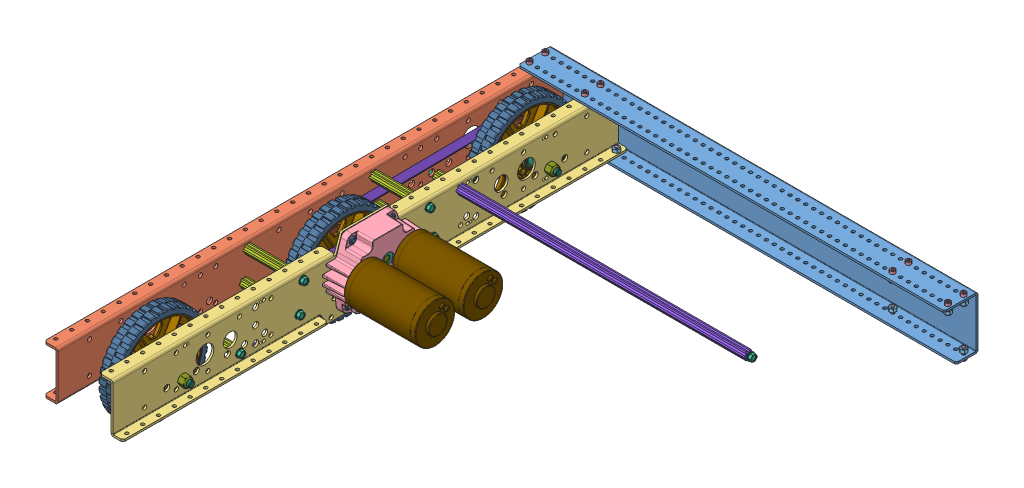
SolidWorks assembly AM14U4 Long Half, configuration Default. Lengths in mm.
Overall size (686.9 159.29 816.74).
156 component instances, 36 part files, 34 mates.
Components (placement in the parent):
- AM14U4 Long Frame Half-1: AM14U4 Long Frame Half [Default] at (226.8656 49.3843 -371.735) size (686.9 116.33 816.74)
  - am-3920 AM14U4 End Plate Long-1: am-3920 AM14U4 End Plate Long [Default] at (-787.4 -81.407 -3.175) x (1 0 0) z (0 -1 0) size (685.8 53.98 84.58)
  - am-3921 AM14U4 Outside Plate-2: am-3921 AM14U4 Outside Plate [Default] at (-666.75 -77.216 813.562) x (0 0 -1) z (0 -1 0) size (812.8 22.23 77.72)
  - am-3922 AM14U4 Inside Plate-1: am-3922 AM14U4 Inside Plate [Default] at (-577.85 -77.216 813.562) x (0 0 -1) z (0 -1 0) size (812.8 38.1 116.33)
  - am-1002 and am-1042 10-32 x 0500 and Nylock Nut Assembly-7: am-1002 and am-1042 10-32 x 0500 and Nylock Nut Assembly [Default] at (-9.8821 -6.6363 9.8132) x (0 -1 0) z (0 0 1) size (17.53 13.8 13)
    - 10-32x0500_shcs-1: 10-32x0500_shcs [HX-SHCS 0.19-32x1.375x1-C] at (-11.4623 3.5321 3.6488) size (17.53 7.94 7.94)
    - 10-32 Nylock Nut 1-1: 10-32 Nylock Nut 1 [90631A411] at (-0.0323 3.5321 3.6488) x (0 0.381849 -0.924225) z (0 -0.924225 -0.381849) size (9.53 6.11 11)
  - am-1002 and am-1042 10-32 x 0500 and Nylock Nut Assembly-8: am-1002 and am-1042 10-32 x 0500 and Nylock Nut Assembly [Default] at (-9.8821 -6.6363 35.2132) x (0 -1 0) z (0 0 1) size (17.53 13.8 13)
    - 10-32x0500_shcs-1: 10-32x0500_shcs [HX-SHCS 0.19-32x1.375x1-C] at (-11.4623 3.5321 3.6488) size (17.53 7.94 7.94)
    - 10-32 Nylock Nut 1-1: 10-32 Nylock Nut 1 [90631A411] at (-0.0323 3.5321 3.6488) x (0 0.381849 -0.924225) z (0 -0.924225 -0.381849) size (9.53 6.11 11)
  - am-1002 and am-1042 10-32 x 0500 and Nylock Nut Assembly-9: am-1002 and am-1042 10-32 x 0500 and Nylock Nut Assembly [Default] at (-2.8179 -77.9457 9.8132) x (0 1 0) z (0 0 1) size (17.53 13.8 13)
    - 10-32x0500_shcs-1: 10-32x0500_shcs [HX-SHCS 0.19-32x1.375x1-C] at (-11.4623 3.5321 3.6488) size (17.53 7.94 7.94)
    - 10-32 Nylock Nut 1-1: 10-32 Nylock Nut 1 [90631A411] at (-0.0323 3.5321 3.6488) x (0 0.381849 -0.924225) z (0 -0.924225 -0.381849) size (9.53 6.11 11)
  - am-1002 and am-1042 10-32 x 0500 and Nylock Nut Assembly-10: am-1002 and am-1042 10-32 x 0500 and Nylock Nut Assembly [Default] at (-98.7821 -6.6363 9.8132) x (0 -1 0) z (0 0 1) size (17.53 13.8 13)
    - 10-32x0500_shcs-1: 10-32x0500_shcs [HX-SHCS 0.19-32x1.375x1-C] at (-11.4623 3.5321 3.6488) size (17.53 7.94 7.94)
    - 10-32 Nylock Nut 1-1: 10-32 Nylock Nut 1 [90631A411] at (-0.0323 3.5321 3.6488) x (0 0.381849 -0.924225) z (0 -0.924225 -0.381849) size (9.53 6.11 11)
  - am-1002 and am-1042 10-32 x 0500 and Nylock Nut Assembly-11: am-1002 and am-1042 10-32 x 0500 and Nylock Nut Assembly [Default] at (-98.7821 -6.6363 35.2132) x (0 -1 0) z (0 0 1) size (17.53 13.8 13)
    - 10-32x0500_shcs-1: 10-32x0500_shcs [HX-SHCS 0.19-32x1.375x1-C] at (-11.4623 3.5321 3.6488) size (17.53 7.94 7.94)
    - 10-32 Nylock Nut 1-1: 10-32 Nylock Nut 1 [90631A411] at (-0.0323 3.5321 3.6488) x (0 0.381849 -0.924225) z (0 -0.924225 -0.381849) size (9.53 6.11 11)
  - am-1002 and am-1042 10-32 x 0500 and Nylock Nut Assembly-12: am-1002 and am-1042 10-32 x 0500 and Nylock Nut Assembly [Default] at (-117.1179 -77.9457 9.8132) x (0 1 0) z (0 0 1) size (17.53 13.8 13)
    - 10-32x0500_shcs-1: 10-32x0500_shcs [HX-SHCS 0.19-32x1.375x1-C] at (-11.4623 3.5321 3.6488) size (17.53 7.94 7.94)
    - 10-32 Nylock Nut 1-1: 10-32 Nylock Nut 1 [90631A411] at (-0.0323 3.5321 3.6488) x (0 0.381849 -0.924225) z (0 -0.924225 -0.381849) size (9.53 6.11 11)
  - FHTS 0.25-20-0.75-1: FHTS 0.25-20-0.75 [FHTS 0.25-20-G-0.75-C] at (-574.675 -59.6687 514.6875) x (-1 0 0) z (0 0.924225 0.381849) size (24.64 12.19 12.19)
  - FHTS 0.25-20-0.75-2: FHTS 0.25-20-0.75 [FHTS 0.25-20-G-0.75-C] at (-574.675 -59.6687 299.6365) x (-1 0 0) z (0 0.924225 0.381849) size (24.64 12.19 12.19)
  - FHTS 0.25-20-0.75-3: FHTS 0.25-20-0.75 [FHTS 0.25-20-G-0.75-C] at (-666.75 -59.6687 299.6365) x (1 0 0) z (0 -0.98696 0.160968) size (24.64 12.19 12.19)
  - FHTS 0.25-20-0.75-4: FHTS 0.25-20-0.75 [FHTS 0.25-20-G-0.75-C] at (-666.75 -59.6687 514.6875) size (24.64 12.19 12.19)
  - FHTS 0.25-20-0.75-5: FHTS 0.25-20-0.75 [FHTS 0.25-20-G-0.75-C] at (-666.75 -65.786 610.362) size (24.64 12.19 12.19)
  - FHTS 0.25-20-0.75-6: FHTS 0.25-20-0.75 [FHTS 0.25-20-G-0.75-C] at (-666.75 -65.786 203.962) size (24.64 12.19 12.19)
  - FHTS 0.25-20-0.75-7: FHTS 0.25-20-0.75 [FHTS 0.25-20-G-0.75-C] at (-574.675 -65.786 203.962) x (-1 0 0) z (0 0.924225 0.381849) size (24.64 12.19 12.19)
  - FHTS 0.25-20-0.75-8: FHTS 0.25-20-0.75 [FHTS 0.25-20-G-0.75-C] at (-574.675 -65.786 610.362) x (-1 0 0) z (0 0.924225 0.381849) size (24.64 12.19 12.19)
  - 3.375in Churro-1: 3.375in Churro [Default] at (-577.85 -65.786 610.362) x (0 0 1) z (-1 0 0) size (14.66 12.7 85.72)
  - 3.375in Churro-2: 3.375in Churro [Default] at (-577.85 -59.6687 514.6875) x (0 0 1) z (-1 0 0) size (14.66 12.7 85.72)
  - 3.375in Churro-3: 3.375in Churro [Default] at (-577.85 -59.6687 299.6365) x (0 0 1) z (-1 0 0) size (14.66 12.7 85.72)
  - 3.375in Churro-4: 3.375in Churro [Default] at (-577.85 -65.786 203.962) x (0 0 1) z (-1 0 0) size (14.66 12.7 85.72)
  - FHTS 0.25-20-0.75-10: FHTS 0.25-20-0.75 [FHTS 0.25-20-G-0.75-C] at (-107.95 -14.986 254.762) x (-1 0 0) z (0 0.924225 0.381849) size (24.64 12.19 12.19)
  - am-1002 and am-1042 10-32 x 0500 and Nylock Nut Assembly-13: am-1002 and am-1042 10-32 x 0500 and Nylock Nut Assembly [Default] at (-682.9821 -6.6363 35.2132) x (0 -1 0) z (0 0 1) size (17.53 13.8 13)
    - 10-32x0500_shcs-1: 10-32x0500_shcs [HX-SHCS 0.19-32x1.375x1-C] at (-11.4623 3.5321 3.6488) size (17.53 7.94 7.94)
    - 10-32 Nylock Nut 1-1: 10-32 Nylock Nut 1 [90631A411] at (-0.0323 3.5321 3.6488) x (0 0.381849 -0.924225) z (0 -0.924225 -0.381849) size (9.53 6.11 11)
  - am-1002 and am-1042 10-32 x 0500 and Nylock Nut Assembly-14: am-1002 and am-1042 10-32 x 0500 and Nylock Nut Assembly [Default] at (-682.9821 -6.6363 9.8132) x (0 -1 0) z (0 0 1) size (17.53 13.8 13)
    - 10-32x0500_shcs-1: 10-32x0500_shcs [HX-SHCS 0.19-32x1.375x1-C] at (-11.4623 3.5321 3.6488) size (17.53 7.94 7.94)
    - 10-32 Nylock Nut 1-1: 10-32 Nylock Nut 1 [90631A411] at (-0.0323 3.5321 3.6488) x (0 0.381849 -0.924225) z (0 -0.924225 -0.381849) size (9.53 6.11 11)
  - am-1002 and am-1042 10-32 x 0500 and Nylock Nut Assembly-15: am-1002 and am-1042 10-32 x 0500 and Nylock Nut Assembly [Default] at (-594.0821 -6.6363 35.2132) x (0 -1 0) z (0 0 1) size (17.53 13.8 13)
    - 10-32x0500_shcs-1: 10-32x0500_shcs [HX-SHCS 0.19-32x1.375x1-C] at (-11.4623 3.5321 3.6488) size (17.53 7.94 7.94)
    - 10-32 Nylock Nut 1-1: 10-32 Nylock Nut 1 [90631A411] at (-0.0323 3.5321 3.6488) x (0 0.381849 -0.924225) z (0 -0.924225 -0.381849) size (9.53 6.11 11)
  - am-1002 and am-1042 10-32 x 0500 and Nylock Nut Assembly-16: am-1002 and am-1042 10-32 x 0500 and Nylock Nut Assembly [Default] at (-594.0821 -6.6363 9.8132) x (0 -1 0) z (0 0 1) size (17.53 13.8 13)
    - 10-32x0500_shcs-1: 10-32x0500_shcs [HX-SHCS 0.19-32x1.375x1-C] at (-11.4623 3.5321 3.6488) size (17.53 7.94 7.94)
    - 10-32 Nylock Nut 1-1: 10-32 Nylock Nut 1 [90631A411] at (-0.0323 3.5321 3.6488) x (0 0.381849 -0.924225) z (0 -0.924225 -0.381849) size (9.53 6.11 11)
  - am-1002 and am-1042 10-32 x 0500 and Nylock Nut Assembly-17: am-1002 and am-1042 10-32 x 0500 and Nylock Nut Assembly [Default] at (-561.6179 -77.9457 9.8132) x (0 1 0) z (0 0 1) size (17.53 13.8 13)
    - 10-32x0500_shcs-1: 10-32x0500_shcs [HX-SHCS 0.19-32x1.375x1-C] at (-11.4623 3.5321 3.6488) size (17.53 7.94 7.94)
    - 10-32 Nylock Nut 1-1: 10-32 Nylock Nut 1 [90631A411] at (-0.0323 3.5321 3.6488) x (0 0.381849 -0.924225) z (0 -0.924225 -0.381849) size (9.53 6.11 11)
  - am-1002 and am-1042 10-32 x 0500 and Nylock Nut Assembly-18: am-1002 and am-1042 10-32 x 0500 and Nylock Nut Assembly [Default] at (-675.9179 -77.9457 9.8132) x (0 1 0) z (0 0 1) size (17.53 13.8 13)
    - 10-32x0500_shcs-1: 10-32x0500_shcs [HX-SHCS 0.19-32x1.375x1-C] at (-11.4623 3.5321 3.6488) size (17.53 7.94 7.94)
    - 10-32 Nylock Nut 1-1: 10-32 Nylock Nut 1 [90631A411] at (-0.0323 3.5321 3.6488) x (0 0.381849 -0.924225) z (0 -0.924225 -0.381849) size (9.53 6.11 11)
  - 18.250in Churro-1: 18.250in Churro [Default] at (-342.9 -14.986 254.762) x (0 0 1) z (-1 0 0) size (14.66 12.7 463.55)
  - FHTS 0.25-20-0.75-11: FHTS 0.25-20-0.75 [FHTS 0.25-20-G-0.75-C] at (-577.85 -14.986 254.762) size (24.64 12.19 12.19)
  - 3.375in Churro-5: 3.375in Churro [Default] at (-663.575 -14.986 305.562) x (0 0.866025 0.5) z (1 0 0) size (14.66 12.7 85.72)
  - FHTS 0.25-20-0.75-12: FHTS 0.25-20-0.75 [FHTS 0.25-20-G-0.75-C] at (-666.75 -14.986 305.562) x (1 0 0) z (0 -0.98696 0.160968) size (24.64 12.19 12.19)
  - FHTS 0.25-20-0.75-14: FHTS 0.25-20-0.75 [FHTS 0.25-20-G-0.75-C] at (-574.675 -14.986 305.562) x (-1 0 0) z (0 0.924225 0.381849) size (24.64 12.19 12.19)
  - FHTS 0.25-20-0.75-15: FHTS 0.25-20-0.75 [FHTS 0.25-20-G-0.75-C] at (-574.675 -14.986 508.762) x (-1 0 0) z (0 0.924225 0.381849) size (24.64 12.19 12.19)
  - 3.375in Churro-6: 3.375in Churro [Default] at (-663.575 -14.986 508.762) x (0 0.866025 0.5) z (1 0 0) size (14.66 12.7 85.72)
  - FHTS 0.25-20-0.75-16: FHTS 0.25-20-0.75 [FHTS 0.25-20-G-0.75-C] at (-666.75 -14.986 508.762) size (24.64 12.19 12.19)
- 6 HiGrip with bearings, pulleys and spacers-1: 6 HiGrip with bearings, pulleys and spacers [Default] at (-425.4709 -83.8657 198.1055) size (85.56 152.4 152.4)
  - 6 HiGrip Asm Rev II-1: 6 HiGrip Asm Rev II [Default] at (83.7987 67.439 110.9939) size (35.05 152.4 152.4)
    - 6 wheel Rev 4-1: 6 wheel Rev 4 [Default] at (-52.6446 9.4231 21.378) size (35.05 132.08 132.08)
    - 6 wheel tread II-1: 6 wheel tread II [Default] at (-65.3446 9.4231 21.378) x (0 0 -1) z (1 0 0) size (152.4 152.4 25.58)
  - 42 tooth HTD Pulley half 2014-1: 42 tooth HTD Pulley half 2014 [Default] at (47.6006 76.862 132.3719) x (1 0 0) z (0 -0.5 0.866025) size (13 74.23 74.23)
  - 42 tooth HTD Pulley half 2014-2: 42 tooth HTD Pulley half 2014 [Default] at (64.263 76.862 132.3719) x (-1 0 0) z (0 -0.499927 0.866067) size (13 74.23 74.23)
  - 1614Z Bearing-1: 1614Z Bearing [Default] at (62.612 76.862 132.3719) x (0 -0.157148 -0.987575) z (-1 0 0) size (28.57 28.57 9.53)
  - 10-24 Hex Washer Rolling x 1.25-1: 10-24 Hex Washer Rolling x 1.25 [93882A213] at (63.247 76.8605 108.5602) x (0 0 -1) z (1 0 0) size (10.52 10.52 35.59)
  - 10-24 Hex Washer Rolling x 1.25-2: 10-24 Hex Washer Rolling x 1.25 [93882A213] at (63.247 97.4833 120.4656) x (0 0 -1) z (1 0 0) size (10.52 10.52 35.59)
  - 10-24 Hex Washer Rolling x 1.25-3: 10-24 Hex Washer Rolling x 1.25 [93882A213] at (63.247 56.2398 144.2799) x (0 0 -1) z (1 0 0) size (10.52 10.52 35.59)
  - 10-24 Hex Washer Rolling x 1.25-4: 10-24 Hex Washer Rolling x 1.25 [93882A213] at (63.247 76.8625 156.1852) x (0 -0.95788 -0.287168) z (1 0 0) size (10.52 10.52 35.59)
  - 10-24 Hex Washer Rolling x 1.25-5: 10-24 Hex Washer Rolling x 1.25 [93882A213] at (63.247 97.4843 144.2781) x (0 -0.868976 0.494854) z (1 0 0) size (10.52 10.52 35.59)
  - 10-24 Hex Washer Rolling x 1.25-6: 10-24 Hex Washer Rolling x 1.25 [93882A213] at (63.247 56.2388 120.4674) x (0 -0.977348 -0.211637) z (1 0 0) size (10.52 10.52 35.59)
  - am-1306 spacer 0280 WashersUSA 13RS052001-1: am-1306 spacer 0280 WashersUSA 13RS052001 [Default] at (74.4865 76.862 132.3719) x (0 -0.35357 0.935408) z (-1 0 0) size (13.16 13.16 7.11)
  - 1614Z Bearing-2: 1614Z Bearing [Default] at (15.2791 76.862 132.3719) x (0 0.155433 -0.987846) z (-1 0 0) size (28.57 28.57 9.53)
  - am-1307 850 long 380 id-1: am-1307 850 long 380 id [Default] at (10.5166 76.862 132.3719) x (0 0.971418 -0.237374) z (0 0.237374 0.971418) size (19.05 21.59 19.05)
- 6 HiGrip with bearings, pulleys and spacers-2: 6 HiGrip with bearings, pulleys and spacers [Default] at (-362.0578 -83.4544 -127.0135) x (-1 0 0) z (0 -0.003104 -0.999995) size (85.56 152.4 152.4)
  - 6 HiGrip Asm Rev II-1: 6 HiGrip Asm Rev II [Default] at (83.7987 67.439 110.9939) size (35.05 152.4 152.4)
    - 6 wheel Rev 4-1: 6 wheel Rev 4 [Default] at (-52.6446 9.4231 21.378) size (35.05 132.08 132.08)
    - 6 wheel tread II-1: 6 wheel tread II [Default] at (-65.3446 9.4231 21.378) x (0 0 -1) z (1 0 0) size (152.4 152.4 25.58)
  - 42 tooth HTD Pulley half 2014-1: 42 tooth HTD Pulley half 2014 [Default] at (47.6006 76.862 132.3719) x (1 0 0) z (0 -0.5 0.866025) size (13 74.23 74.23)
  - 42 tooth HTD Pulley half 2014-2: 42 tooth HTD Pulley half 2014 [Default] at (64.263 76.862 132.3719) x (-1 0 0) z (0 -0.499927 0.866067) size (13 74.23 74.23)
  - 1614Z Bearing-1: 1614Z Bearing [Default] at (62.612 76.862 132.3719) x (0 -0.157148 -0.987575) z (-1 0 0) size (28.57 28.57 9.53)
  - 10-24 Hex Washer Rolling x 1.25-1: 10-24 Hex Washer Rolling x 1.25 [93882A213] at (63.247 76.8605 108.5602) x (0 0 -1) z (1 0 0) size (10.52 10.52 35.59)
  - 10-24 Hex Washer Rolling x 1.25-2: 10-24 Hex Washer Rolling x 1.25 [93882A213] at (63.247 97.4833 120.4656) x (0 0 -1) z (1 0 0) size (10.52 10.52 35.59)
  - 10-24 Hex Washer Rolling x 1.25-3: 10-24 Hex Washer Rolling x 1.25 [93882A213] at (63.247 56.2398 144.2799) x (0 0 -1) z (1 0 0) size (10.52 10.52 35.59)
  - 10-24 Hex Washer Rolling x 1.25-4: 10-24 Hex Washer Rolling x 1.25 [93882A213] at (63.247 76.8625 156.1852) x (0 -0.95788 -0.287168) z (1 0 0) size (10.52 10.52 35.59)
  - 10-24 Hex Washer Rolling x 1.25-5: 10-24 Hex Washer Rolling x 1.25 [93882A213] at (63.247 97.4843 144.2781) x (0 -0.868976 0.494854) z (1 0 0) size (10.52 10.52 35.59)
  - 10-24 Hex Washer Rolling x 1.25-6: 10-24 Hex Washer Rolling x 1.25 [93882A213] at (63.247 56.2388 120.4674) x (0 -0.977348 -0.211637) z (1 0 0) size (10.52 10.52 35.59)
  - am-1306 spacer 0280 WashersUSA 13RS052001-1: am-1306 spacer 0280 WashersUSA 13RS052001 [Default] at (74.4865 76.862 132.3719) x (0 -0.35357 0.935408) z (-1 0 0) size (13.16 13.16 7.11)
  - 1614Z Bearing-2: 1614Z Bearing [Default] at (15.2791 76.862 132.3719) x (0 0.155433 -0.987846) z (-1 0 0) size (28.57 28.57 9.53)
  - am-1307 850 long 380 id-1: am-1307 850 long 380 id [Default] at (10.5166 76.862 132.3719) x (0 0.971418 -0.237374) z (0 0.237374 0.971418) size (19.05 21.59 19.05)
- am-2598_107 2016 KOP Toughbox Mini-1: am-2598_107 2016 KOP Toughbox Mini [Default] at (-398.3511 -20.6298 126.5278) x (0 0.001296 0.999999) z (-1 0 0) size (140.05 121.81 142.29)
  - Toughbox d07-1: Toughbox d07 [Default] at (-88.5589 93.4503 -52.3959) x (-0.336928 0.94153 0) z (0.94153 0.336928 0) size (11 38.23 9.52)
  - Toughbox d05-1: Toughbox d05 [Default] at (-91.0349 50.9043 -67.5597) x (-0.336928 0.94153 0) z (0 0 -1) size (65.97 66.04 10.16)
  - FR6ZZ Bearing-1: FR6ZZ Bearing [Default] at (-96.247 60.278 -52.5991) x (-0.893862 0.448342 0) z (0 0 1) size (24.69 24.69 7.16)
  - 10-32 Nylock Nut-1: 10-32 Nylock Nut [Default] at (-129.8464 -8.0737 -56.3837) x (0.501678 0.865055 0) z (0 0 -1) size (10.18 11.01 7.1)
  - 10-32 Nylock Nut-2: 10-32 Nylock Nut [Default] at (-59.2462 80.7349 -56.3837) x (0.999999 -0.001296 0) z (0 0 -1) size (10.18 11.01 7.1)
  - 10-32 Nylock Nut-3: 10-32 Nylock Nut [Default] at (-122.7461 80.8172 -56.3837) x (0.500567 0.865698 0) z (0 0 -1) size (10.18 11.01 7.1)
  - 10-32 Nylock Nut-4: 10-32 Nylock Nut [Default] at (-52.3764 -8.1741 -56.3837) x (-0.501678 -0.865055 0) z (0 0 -1) size (10.18 11.01 7.1)
  - 5-16 washer-1: 5-16 washer [Default] at (-52.3162 38.3079 -77.7705) x (0.38418 -0.923258 0) z (0 0 -1) size (17.53 17.53 1.47)
  - 5-16 washer-2: 5-16 washer [Default] at (-52.3162 38.3079 -76.2973) x (0.897267 -0.441488 0) z (0 0 -1) size (17.53 17.53 1.47)
  - 5-16 washer-3: 5-16 washer [Default] at (-129.7861 38.4083 -77.7705) x (-0.990116 0.140253 0) z (0 0 1) size (17.53 17.53 1.47)
  - 5-16 washer-4: 5-16 washer [Default] at (-129.7861 38.4083 -79.2437) x (-0.681761 0.731575 0) z (0 0 1) size (17.53 17.53 1.47)
  - Toughbox d09-1: Toughbox d09 [Default] at (-52.3162 38.3079 -63.5973) x (0.910249 -0.414061 0) z (0 0 -1) size (20.03 20.32 12.7)
  - Toughbox d09-2: Toughbox d09 [Default] at (-129.7861 38.4083 -63.5973) x (0.075368 -0.997156 0) z (0 0 -1) size (20.03 20.32 12.7)
  - TM Housing-1: TM Housing [Default] at (-91.0876 10.1882 -86.3557) x (0.999999 -0.001296 0) z (0 0 1) size (139.9 118.55 41.54)
  - SHCS 10-32 x 0.625-1: SHCS 10-32 x 0.625 [Default] at (-52.2832 63.7078 -74.4685) x (-0.564778 -0.825243 0) z (-0.825243 0.564778 0) size (7.82 20.65 7.82)
  - SHCS 10-32 x 0.625-2: SHCS 10-32 x 0.625 [Default] at (-122.7461 80.8172 -42.5915) x (0.507484 -0.861661 0) z (-0.861661 -0.507484 0) size (7.82 20.65 7.82)
  - SHCS 10-32 x 0.625-3: SHCS 10-32 x 0.625 [Default] at (-52.3764 -8.1741 -42.5915) x (0.507484 -0.861661 0) z (-0.861661 -0.507484 0) size (7.82 20.65 7.82)
  - SHCS 10-32 x 0.625-4: SHCS 10-32 x 0.625 [Default] at (-129.8464 -8.0737 -42.5915) x (0.507484 -0.861661 0) z (-0.861661 -0.507484 0) size (7.82 20.65 7.82)
  - SHCS 10-32 x 0.625-5: SHCS 10-32 x 0.625 [Default] at (-59.2462 80.7349 -42.5915) x (0.740711 -0.671824 0) z (-0.671824 -0.740711 0) size (7.82 20.65 7.82)
  - SHCS 10-32 x 0.625-6: SHCS 10-32 x 0.625 [Default] at (-52.3491 12.9079 -74.4685) x (-0.564778 -0.825243 0) z (-0.825243 0.564778 0) size (7.82 20.65 7.82)
  - SHCS 10-32 x 0.625-7: SHCS 10-32 x 0.625 [Default] at (-129.7532 63.8083 -74.4685) x (-0.966277 -0.257503 0) z (-0.257503 0.966277 0) size (7.82 20.65 7.82)
  - SHCS 10-32 x 0.625-8: SHCS 10-32 x 0.625 [Default] at (-129.819 13.0083 -74.4685) x (-0.99652 0.083357 0) z (0.083357 0.99652 0) size (7.82 20.65 7.82)
  - R6ZZ Bearing-3: R6ZZ Bearing [Default] at (-91.0349 50.9043 -84.8317) x (0.958138 -0.286306 0) z (0 0 1) size (22.23 22.23 7.11)
  - R6ZZ Bearing-4: R6ZZ Bearing [Default] at (-91.0876 10.1882 -84.8317) x (-0.328282 -0.94458 0) z (0 0 1) size (22.23 22.23 7.11)
  - 8mm spring clip-1: 8mm spring clip [Default] at (-129.7861 38.4083 -63.5973) x (0 0 1) z (-1 0 0) size (1.09 14.83 14.83)
  - 8mm spring clip-2: 8mm spring clip [Default] at (-52.3162 38.3079 -63.5973) x (0 0 1) z (-1 0 0) size (1.09 14.83 14.83)
  - 500 E-klip-1: 500 E-klip [Default] at (-91.0876 10.1882 -64.4355) x (0.996411 -0.084651 0) z (0 0 1) size (19.07 20.96 1.27)
  - FR8ZZ Hex Bearing-1: FR8ZZ Hex Bearing [Default] at (-91.0876 10.1882 -44.6717) x (-0.5 0.866025 0) z (0 0 -1) size (31.12 31.12 7.93)
  - 16t 20dp 375h with teeth-1: 16t 20dp 375h with teeth [Default] at (-91.0349 50.9043 -67.5597) x (0 0 1) z (-0.983853 0.178977 0) size (15.19 22.57 22.57)
  - 48t 20dp 500h with teeth-1: 48t 20dp 500h with teeth [Default] at (-91.0876 10.1882 -63.1655) x (0 0 1) z (-1 0 0) size (10.21 63.42 63.42)
  - TB Output Shaft Hex L-Base 2-1: TB Output Shaft Hex L-Base 2 [Default] at (-52.7805 -6.4809 -52.3197) x (1 0 0) z (0 -1 0) size (14.66 142.29 12.7)
- FR8ZZ Hex Bearing-2: FR8ZZ Hex Bearing [Default] at (-443.1127 -10.5597 35.427) x (0 -0.866673 -0.498877) z (1 0 0) size (31.12 31.12 7.93)
- 6 HiGrip with hub and double pulley-1: 6 HiGrip with hub and double pulley [Default] at (-361.9841 -87.2508 167.898) x (-1 0 0) z (0 -0.001296 -0.999999) size (81.42 152.4 152.4)
  - 6 HiGrip Asm Rev II-1: 6 HiGrip Asm Rev II [Default] at (83.7987 67.439 110.9939) size (35.05 152.4 152.4)
    - 6 wheel Rev 4-1: 6 wheel Rev 4 [Default] at (-52.6446 9.4231 21.378) size (35.05 132.08 132.08)
    - 6 wheel tread II-1: 6 wheel tread II [Default] at (-65.3446 9.4231 21.378) x (0 0 -1) z (1 0 0) size (152.4 152.4 25.58)
  - 42 tooth HTD Pulley half 2014-1: 42 tooth HTD Pulley half 2014 [Default] at (47.6006 76.862 132.3719) x (1 0 0) z (0 -0.5 0.866025) size (13 74.23 74.23)
  - 42 tooth HTD Pulley half 2014-2: 42 tooth HTD Pulley half 2014 [Default] at (64.263 76.862 132.3719) x (-1 0 0) z (0 -0.499927 0.866067) size (13 74.23 74.23)
  - 10-24 Hex Washer Rolling x 1.25-1: 10-24 Hex Washer Rolling x 1.25 [93882A213] at (63.247 76.8605 108.5602) x (0 0 -1) z (1 0 0) size (10.52 10.52 35.59)
  - 10-24 Hex Washer Rolling x 1.25-2: 10-24 Hex Washer Rolling x 1.25 [93882A213] at (63.247 97.4833 120.4656) x (0 0 -1) z (1 0 0) size (10.52 10.52 35.59)
  - 10-24 Hex Washer Rolling x 1.25-3: 10-24 Hex Washer Rolling x 1.25 [93882A213] at (63.247 56.2398 144.2799) x (0 0 -1) z (1 0 0) size (10.52 10.52 35.59)
  - 10-24 Hex Washer Rolling x 1.25-4: 10-24 Hex Washer Rolling x 1.25 [93882A213] at (63.247 76.8625 156.1852) x (0 -0.95788 -0.287168) z (1 0 0) size (10.52 10.52 35.59)
  - 10-24 Hex Washer Rolling x 1.25-5: 10-24 Hex Washer Rolling x 1.25 [93882A213] at (63.247 97.4843 144.2781) x (0 -0.868976 0.494854) z (1 0 0) size (10.52 10.52 35.59)
  - 10-24 Hex Washer Rolling x 1.25-6: 10-24 Hex Washer Rolling x 1.25 [93882A213] at (63.247 56.2388 120.4674) x (0 -0.748729 -0.662876) z (1 0 0) size (10.52 10.52 35.59)
  - 42 tooth HTD Pulley half 2014-3: 42 tooth HTD Pulley half 2014 [Default] at (-1.9548 76.8628 132.3714) x (1 0 0) z (0 -1 -0.000063) size (13 74.23 74.23)
  - 42 tooth HTD Pulley half 2014-4: 42 tooth HTD Pulley half 2014 [Default] at (14.7076 76.8628 132.3714) x (-1 0 0) z (0 -1 0.000021) size (13 74.23 74.23)
  - 500EX Hex Hub-1: 500EX Hex Hub [Default] at (-8.3048 76.8628 132.3714) x (0 -0.866025 -0.5) z (0 -0.5 0.866025) size (55.37 25.4 51.33)
  - 10-24 Hex Washer Rolling x 1.25-7: 10-24 Hex Washer Rolling x 1.25 [93882A213] at (-5.2568 97.485 120.4652) x (0 0 1) z (-1 0 0) size (10.52 10.52 35.59)
  - 10-24 Hex Washer Rolling x 1.25-8: 10-24 Hex Washer Rolling x 1.25 [93882A213] at (-5.2568 76.8628 108.5589) x (0 0 1) z (-1 0 0) size (10.52 10.52 35.59)
  - 10-24 Hex Washer Rolling x 1.25-9: 10-24 Hex Washer Rolling x 1.25 [93882A213] at (-5.2568 56.2406 120.4652) x (0 0 1) z (-1 0 0) size (10.52 10.52 35.59)
  - 10-24 Hex Washer Rolling x 1.25-10: 10-24 Hex Washer Rolling x 1.25 [93882A213] at (-5.2568 97.485 144.2777) x (0 -0.99374 -0.111715) z (-1 0 0) size (10.52 10.52 35.59)
  - 10-24 Hex Washer Rolling x 1.25-11: 10-24 Hex Washer Rolling x 1.25 [93882A213] at (-5.2568 56.2406 144.2777) x (0 -0.138911 0.990305) z (-1 0 0) size (10.52 10.52 35.59)
  - 10-24 Hex Washer Rolling x 1.25-12: 10-24 Hex Washer Rolling x 1.25 [93882A213] at (-5.2568 76.8628 156.1839) x (0 -0.98811 -0.15375) z (-1 0 0) size (10.52 10.52 35.59)
  - am-1305 500 Hex Spacer-1: am-1305 500 Hex Spacer [Default] at (57.8495 76.862 132.3719) x (0 -0.866025 -0.5) z (0 -0.5 0.866025) size (28.55 14.48 28.55)
- 375-16 x 4.25 Hex Bolt-1: 375-16 x 4.25 Hex Bolt [HFBOLT 0.375-16x2.5x1-C] at (-446.0566 -7.0037 330.4774) size (114.12 16.48 14.27)
- 375-16 x 4.25 Hex Bolt-2: 375-16 x 4.25 Hex Bolt [HFBOLT 0.375-16x2.5x1-C] at (-446.0566 -7.0037 -259.6233) size (114.12 16.48 14.27)
- 375-16 Lock Nut-1: 375-16 Lock Nut [91831A127] at (-347.8094 -7.0037 330.4774) x (0 -1 0) z (0 0 1) size (14.29 12 16.5)
- 375-16 Lock Nut-2: 375-16 Lock Nut [91831A127] at (-347.8094 -7.0037 -259.6233) x (0 -1 0) z (0 0 1) size (14.29 12 16.5)
- 800-5M-15 v2-1: 800-5M-15 v2 [Default] at (-376.6917 -7.0037 330.4774) x (0 -0.012051 -0.999927) z (0 -0.999927 0.012051) size (368.15 15 73.08)
- 800-5M-15 v2-2: 800-5M-15 v2 [Default] at (-409.5847 -7.0037 -259.6233) x (0 -0.012051 0.999927) z (0 -0.999927 -0.012051) size (368.15 15 73.08)
- CIM Motor SW-1: CIM Motor SW [Default] at (-292.9454 -17.9498 105.9882) x (0 1 0) z (-1 0 0) size (64.01 64.01 154.93)
- CIM Motor SW-2: CIM Motor SW [Default] at (-292.9454 -17.9498 183.4582) x (0 1 0) z (-1 0 0) size (64.01 64.01 154.93)
Mates (geometry in assembly coordinates):
- Coincident1: coincident: plane of AM14U4 Long Frame Half-1/am-3922 AM14U4 Inside Plate-1 through (-350.9844 42.0183 441.827) normal (-1 0 0); plane of 6 HiGrip with bearings, pulleys and spacers-1/am-1306 spacer 0280 WashersUSA 13RS052001-1 through (-350.9844 -7.0037 330.4774) normal (1 0 0)
- Concentric1: concentric: cylinder of AM14U4 Long Frame Half-1/am-3922 AM14U4 Inside Plate-1 through (-370.0344 -7.0037 330.4774) axis (1 0 0) radius 4.826; cylinder of 6 HiGrip with bearings, pulleys and spacers-1/am-1306 spacer 0280 WashersUSA 13RS052001-1 through (-358.0964 -7.0037 330.4774) axis (1 0 0) radius 4.8514
- Coincident2: coincident: plane of AM14U4 Long Frame Half-1/am-3922 AM14U4 Inside Plate-1 through (-350.9844 42.0183 441.827) normal (-1 0 0); plane of 6 HiGrip with bearings, pulleys and spacers-2/am-1307 850 long 380 id-1 through (-350.9844 -7.0037 -259.6233) normal (1 0 0)
- Concentric2: concentric: cylinder of AM14U4 Long Frame Half-1/am-3922 AM14U4 Inside Plate-1 through (-370.0344 -7.0037 -259.6233) axis (1 0 0) radius 4.826; cylinder of 6 HiGrip with bearings, pulleys and spacers-2/am-1307 850 long 380 id-1 through (-350.9844 -7.0037 -259.6233) axis (-1 0 0) radius 9.525
- Concentric3: concentric: cylinder of AM14U4 Long Frame Half-1/am-3922 AM14U4 Inside Plate-1 through (-350.9844 -10.5597 35.427) axis (1 0 0) radius 14.2875; cylinder of am-2598_107 2016 KOP Toughbox Mini-1/FR8ZZ Hex Bearing-1 through (-345.752 -10.5597 35.427) axis (-1 0 0) radius 14.2875
- Parallel1: parallel: plane of AM14U4 Long Frame Half-1/am-3922 AM14U4 Inside Plate-1 through (-347.8094 69.4503 -12.198) normal (0 1 0); line of am-2598_107 2016 KOP Toughbox Mini-1/TM Housing-1 through (-347.2837 69.0075 3.677) axis (0 0 1)
- Coincident4: coincident: plane of AM14U4 Long Frame Half-1/am-3922 AM14U4 Inside Plate-1 through (-347.8094 42.0183 441.827) normal (1 0 0); plane of am-2598_107 2016 KOP Toughbox Mini-1/TM Housing-1 through (-347.8094 -10.5597 35.427) normal (-1 0 0)
- Coincident51: coincident: plane of AM14U4 Long Frame Half-1/am-3921 AM14U4 Outside Plate-2 through (-363.6844 -28.5937 -370.973) normal (0 1 0); plane of ? through (-278.8772 -28.5937 102.9513) normal (0 -1 0)
- Concentric41: concentric: cylinder of AM14U4 Long Frame Half-1/am-3921 AM14U4 Outside Plate-2 through (-439.8844 -10.5597 35.427) axis (1 0 0) radius 14.2875; cylinder of FR8ZZ Hex Bearing-2 through (-435.1854 -10.5597 35.427) axis (-1 0 0) radius 13.97
- Coincident61: coincident: plane of AM14U4 Long Frame Half-1/am-3921 AM14U4 Outside Plate-2 through (-436.7094 42.0183 441.827) normal (1 0 0); plane of FR8ZZ Hex Bearing-2 through (-436.7094 -22.6671 28.4577) normal (-1 0 0)
- Coincident7: coincident: plane of am-2598_107 2016 KOP Toughbox Mini-1/TB Output Shaft Hex L-Base 2-1 through (-320.6314 -10.5692 28.0947) normal (0 -0.501122 -0.865376); plane of FR8ZZ Hex Bearing-2 through (-435.1854 -10.5692 28.0947) normal (0 0.501122 0.865376)
- Concentric5: concentric: cylinder of am-2598_107 2016 KOP Toughbox Mini-1/FR8ZZ Hex Bearing-1 through (-345.752 -10.5597 35.427) axis (-1 0 0) radius 14.2875; circle of 6 HiGrip with hub and double pulley-1/500EX Hex Hub-1
- Parallel2: parallel: plane of am-2598_107 2016 KOP Toughbox Mini-1/TB Output Shaft Hex L-Base 2-1 through (-320.6314 -10.5502 42.7594) normal (0 0.501122 0.865376); plane of 6 HiGrip with hub and double pulley-1/500EX Hex Hub-1 through (-353.6793 -10.5692 28.08) normal (0 0.501122 0.865376)
- Coincident9: coincident: plane of am-2598_107 2016 KOP Toughbox Mini-1/FR8ZZ Hex Bearing-1 through (-353.6793 -10.5597 35.427) normal (-1 0 0); plane of 6 HiGrip with hub and double pulley-1/500EX Hex Hub-1 through (-353.6793 -10.5597 35.427) normal (1 0 0)
- Concentric61: concentric: cylinder of AM14U4 Long Frame Half-1/am-3921 AM14U4 Outside Plate-2 through (-547.8354 -7.0037 330.4774) axis (1 0 0) radius 4.826; cylinder of 375-16 x 4.25 Hex Bolt-1 through (-446.0566 -7.0037 330.4774) axis (-1 0 0) radius 7.1374
- Coincident101: coincident: plane of AM14U4 Long Frame Half-1/am-3921 AM14U4 Outside Plate-2 through (-439.8844 42.0183 441.827) normal (-1 0 0); plane of 375-16 x 4.25 Hex Bolt-1 through (-439.8844 1.2379 330.4774) normal (1 0 0)
- Concentric71: concentric: cylinder of AM14U4 Long Frame Half-1/am-3921 AM14U4 Outside Plate-2 through (-547.8354 -7.0037 -259.6233) axis (1 0 0) radius 4.826; cylinder of 375-16 x 4.25 Hex Bolt-2 through (-446.0566 -7.0037 -259.6233) axis (-1 0 0) radius 7.1374
- Coincident111: coincident: plane of AM14U4 Long Frame Half-1/am-3921 AM14U4 Outside Plate-2 through (-439.8844 42.0183 441.827) normal (-1 0 0); plane of 375-16 x 4.25 Hex Bolt-2 through (-439.8844 1.2379 -259.6233) normal (1 0 0)
- Coincident12: coincident: plane of AM14U4 Long Frame Half-1/am-3922 AM14U4 Inside Plate-1 through (-347.8094 42.0183 441.827) normal (1 0 0); plane of 375-16 Lock Nut-1 through (-347.8094 0.14 318.1041) normal (-1 0 0)
- Coincident13: coincident: plane of AM14U4 Long Frame Half-1/am-3922 AM14U4 Inside Plate-1 through (-347.8094 42.0183 441.827) normal (1 0 0); plane of 375-16 Lock Nut-2 through (-347.8094 0.14 -271.9967) normal (-1 0 0)
- Concentric8: concentric: cylinder of 375-16 x 4.25 Hex Bolt-2 through (-446.0566 -7.0037 -259.6233) axis (-1 0 0) radius 4.7625; cylinder of 375-16 Lock Nut-2 through (-338.142 -7.0037 -259.6233) axis (-1 0 0) radius 4.0291
- Concentric9: concentric: cylinder of 375-16 x 4.25 Hex Bolt-1 through (-446.0566 -7.0037 330.4774) axis (-1 0 0) radius 4.7625; cylinder of 375-16 Lock Nut-1 through (-338.142 -7.0037 330.4774) axis (-1 0 0) radius 4.0291
- Concentric10: concentric: cylinder of 6 HiGrip with bearings, pulleys and spacers-1/am-1307 850 long 380 id-1 through (-436.5443 -7.0037 330.4774) axis (1 0 0) radius 9.525; cylinder of 800-5M-15 v2-1 through (-361.6917 -7.0037 330.4774) axis (-1 0 0) radius 35.0139
- Concentric11: concentric: cylinder of 6 HiGrip with bearings, pulleys and spacers-2/am-1307 850 long 380 id-1 through (-350.9844 -7.0037 -259.6233) axis (-1 0 0) radius 9.525; cylinder of 800-5M-15 v2-2 through (-424.5847 -7.0037 -259.6233) axis (1 0 0) radius 35.0139
- Concentric12: concentric: circle of AM14U4 Long Frame Half-1/am-3921 AM14U4 Outside Plate-2; cylinder of 800-5M-15 v2-1 through (-361.6917 -10.5597 35.427) axis (-1 0 0) radius 35.0139
- Concentric13: concentric: cylinder of FR8ZZ Hex Bearing-2 through (-435.1854 -10.5597 35.427) axis (-1 0 0) radius 14.2875; cylinder of 800-5M-15 v2-2 through (-424.5847 -10.5597 35.427) axis (1 0 0) radius 35.0139
- Coincident14: coincident: plane of 6 HiGrip with hub and double pulley-1/42 tooth HTD Pulley half 2014-1 through (-409.5847 -10.5605 35.4266) normal (-1 0 0); plane of 800-5M-15 v2-2 through (-409.5847 -7.0037 -259.6233) normal (1 0 0)
- Coincident15: coincident: plane of 6 HiGrip with hub and double pulley-1/42 tooth HTD Pulley half 2014-4 through (-376.6917 -10.5597 35.427) normal (1 0 0); plane of 800-5M-15 v2-1 through (-376.6917 -7.0037 330.4774) normal (-1 0 0)
- Coincident16: coincident: plane of CIM Motor SW-1 through (-311.9954 17.6102 -3.308) normal (-1 0 0); plane of CIM Motor SW-2 through (-311.9954 17.6102 74.162) normal (-1 0 0)
- Concentric14: concentric: cylinder of am-2598_107 2016 KOP Toughbox Mini-1/TM Housing-1 through (-347.8094 17.6102 74.162) axis (-1 0 0) radius 10.414; cylinder of CIM Motor SW-2 through (-303.7658 17.6102 74.162) axis (1 0 0) radius 32.004
- Concentric15: concentric: cylinder of am-2598_107 2016 KOP Toughbox Mini-1/TM Housing-1 through (-347.8094 17.6102 -3.308) axis (-1 0 0) radius 10.414; cylinder of CIM Motor SW-1 through (-303.7658 17.6102 -3.308) axis (1 0 0) radius 32.004
- Concentric16: concentric: cylinder of am-2598_107 2016 KOP Toughbox Mini-1/SHCS 10-32 x 0.625-1 through (-303.2324 43.0102 74.162) axis (-1 0 0) radius 2.3876; cylinder of CIM Motor SW-2 through (-311.9954 43.0102 74.162) axis (-1 0 0) radius 2.0193
- Concentric17: concentric: cylinder of am-2598_107 2016 KOP Toughbox Mini-1/SHCS 10-32 x 0.625-7 through (-303.2324 43.0102 -3.308) axis (-1 0 0) radius 2.3876; cylinder of CIM Motor SW-1 through (-311.9954 43.0102 -3.308) axis (-1 0 0) radius 2.0193
- Coincident17: coincident: plane of am-2598_107 2016 KOP Toughbox Mini-1/TM Housing-1 through (-311.9954 -10.5597 35.427) normal (1 0 0); plane of CIM Motor SW-1 through (-311.9954 17.6102 -3.308) normal (-1 0 0)
